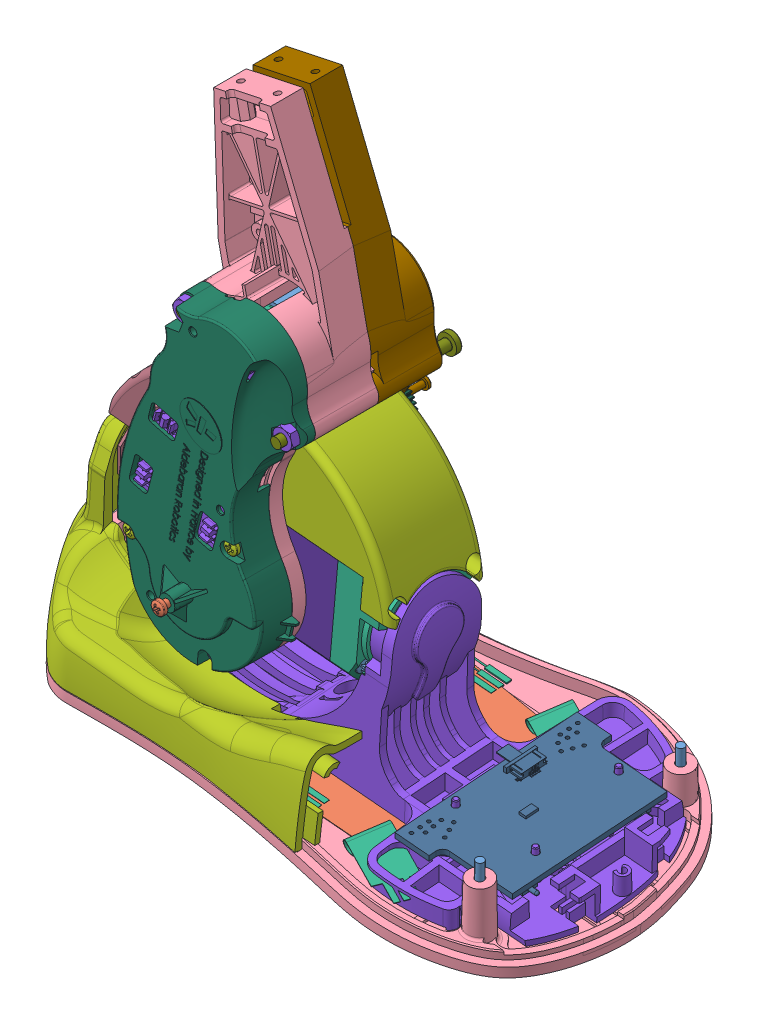
SolidWorks assembly Tibia_gauche, configuration Défaut. Lengths in mm.
Overall size (176.95 174.24 110.8).
97 component instances, 51 part files, 74 mates.
Components (placement in the parent):
- STD_M700013__PZ99_KA22x5_KA22 x 6-1: STD_M700013__PZ99_KA22x5_KA22 x 6 [Default] at (16.9636 -10.9615 1.7353) x (0 0 1) z (0.337513 -0.941321 0) size (6.5 3.9 3.91)
- STD_M700003__PZ99_KA22x6_KA22 x 6-1: STD_M700003__PZ99_KA22x6_KA22 x 6 [Default] at (2.1457 -91.3172 43.0853) x (0 0 -1) z (0.448628 -0.893719 0) size (7.5 3.9 3.91)
- ALD_M010013__P_mobile_inf_1_A00-1: ALD_M010013__P_mobile_inf_1_A00 [Default] at (6.6023 -47.3511 -13.8647) x (-0.555489 0.831524 0) z (-0.831524 -0.555489 0) size (24.51 6.7 24.51)
- ALD_M010048__P_couvercle_tibia_meca_gauche_Axx-1: ALD_M010048__P_couvercle_tibia_meca_gauche_Axx [Default] at (2.8538 9.7275 -12.4647) x (0 -1 0) z (0 0 1) size (91.48 47.32 23.1) (hidden)
- ALD_M010046__P_boitier_tibia_elec_gauche_ALD_M010046__PAxx_boitier_elec_gauche-1: ALD_M010046__P_boitier_tibia_elec_gauche_ALD_M010046__PAxx_boitier_elec_gauche [Default] at (2.8538 9.7275 5.2353) x (0 -1 0) z (0 0 1) size (135.22 47.39 29.9)
- STD_M700013__PZ99_KA22x5_KA22 x 6-2: STD_M700013__PZ99_KA22x5_KA22 x 6 [Default] at (-1.6212 -14.9118 1.7353) x (0 0 1) z (-0.935228 -0.354047 0) size (6.5 3.9 3.91)
- STD_M710004__P_vis_M2x5_ALD_M710004__PZ99_vis_M2x5-1: STD_M710004__P_vis_M2x5_ALD_M710004__PZ99_vis_M2x5 [Default] at (10.4845 -27.6822 -14.6647) x (0 0 1) z (0.702902 0.711287 0) size (6.41 3.8 3.8)
- ALD_M840031-1: ALD_M840031 [Default] at (12.0374 -33.4777 18.7353) x (-0.707107 -0.707107 0) z (0.707107 -0.707107 0) size (22 50.65 22)
- STD_M700005__PZ99_KA22x12_Default-1: STD_M700005__PZ99_KA22x12_Default [Default] at (14.3538 -74.4725 34.0353) x (0 0 -1) z (0.975434 -0.220294 0) size (13.5 3.9 3.91)
- STD_M710004__P_vis_M2x5_ALD_M710004__PZ99_vis_M2x5-2: STD_M710004__P_vis_M2x5_ALD_M710004__PZ99_vis_M2x5 [Default] at (17.8329 -35.0307 -14.6647) x (0 0 1) z (0.331606 0.943418 0) size (6.41 3.8 3.8)
- ALD_E000183__P_Left_Tibia_Card_Default-1: ALD_E000183__P_Left_Tibia_Card_Default [Default] at (-4.5707 -75.2219 31.3353) x (-0.250739 -0.968055 0) z (0 0 1) size (56.57 25 8.51)
- STD_M700006__PZ99_KA18x6_Default-1: STD_M700006__PZ99_KA18x6_Default [Default] at (-0.8831 -76.2311 -39.0647) x (0 0 1) z (0.79364 0.608388 0) size (7.2 3.2 3.2)
- STD_M510004__P_palier_GFM_1517-05_stabdard-1: STD_M510004__P_palier_GFM_1517-05_stabdard [Default] at (2.8538 -90.2725 -9.0647) x (0 0 -1) z (0.822457 -0.568828 0) size (5 23 23)
- ALD_M100068__P_Pinion_inf_4_A00-1: ALD_M100068__P_Pinion_inf_4_A00 [Default] at (-2.245 -74.58 -24.3647) x (0.042959 -0.999077 0) z (-0.999077 -0.042959 0) size (8.58 10.5 8.96)
- ALD_M010289__P_Inf_Limiter_Default-1: ALD_M010289__P_Inf_Limiter_Default [Default] at (-2.245 -74.58 -24.4647) x (0.999077 0.042959 0) z (0 0 1) size (16.14 19.2 3.9)
- STD_M510004__P_palier_GFM_1517-05_stabdard-2: STD_M510004__P_palier_GFM_1517-05_stabdard [Default] at (2.8538 -90.2725 19.5353) x (0 0 1) z (-0.611916 -0.790923 0) size (5 23 23)
- ALD_E000030__P_carte_MRE-1: ALD_E000030__P_carte_MRE [Default] at (-7.1462 -100.2725 30.9353) x (0 1 0) z (0 0 -1) size (18.94 18.94 5)
- ALD_M100018__P_axe_3x20_2-1: ALD_M100018__P_axe_3x20_2 [Default] at (-2.245 -74.58 -29.5647) x (-0.898721 -0.43852 0) z (0 0 1) size (3 3 20)
- ALD_M010050__P_couvercle_tibia_elec_gauche_Axx-1: ALD_M010050__P_couvercle_tibia_elec_gauche_Axx [Default] at (3.2067 9.6772 24.5353) x (-0.010505 -0.999945 0) z (0 0 1) size (91.58 50.24 17.3)
- STD_M700005__PZ99_KA22x12_Default-2: STD_M700005__PZ99_KA22x12_Default [Default] at (-15.1462 -84.8725 -22.6647) x (0 0 1) z (-0.865979 -0.500081 0) size (13.5 3.9 3.91)
- STD_M710005__PZ99_Vis_M3x50_ISO 7045 - M3 x 50-1: STD_M710005__PZ99_Vis_M3x50_ISO 7045 - M3 x 50 [Default] at (-1.7576 -23.8893 -20.5647) x (0 0 1) z (0.06312 0.998006 0) size (52.4 5.6 5.68)
- ALD_M010014__P_mobile_inf_2_A00-1: ALD_M010014__P_mobile_inf_2_A00 [Default] at (1.2276 -60.6565 -18.3647) x (0.438964 -0.898505 0) z (0.898505 0.438964 0) size (19.63 8.2 19.62)
- Left_Foot_jambe droite-1: Left_Foot_jambe droite [Défaut] at (4.3479 -90.4053 5.2353) x (-0.007082 -0.079671 0.996796) z (-0.996073 0.088539 0) size (106.44 58.7 171.69)
  - STD_M850001__P_Scotch_double_Face_3M_5419_Default-1: STD_M850001__P_Scotch_double_Face_3M_5419_Default [Default] at (-23.9002 -40.8442 -61.9998) x (0 0 -1) z (0 1 0) size (13 10 0.25)
  - STD_M700004__PZ99_KA22x8_KA22 x 8-1: STD_M700004__PZ99_KA22x8_KA22 x 8 [Default] at (-16.4 -30.0842 45.1) x (0 1 0) z (-0.943584 0 -0.331134) size (9.5 3.9 3.91)
  - STD_M850001__P_Scotch_double_Face_3M_5419_Default-2: STD_M850001__P_Scotch_double_Face_3M_5419_Default [Default] at (27.1002 -40.5942 -74.9998) x (0 0 1) z (0 -1 0) size (13 10 0.25)
  - STD_E990013__P_FSR_4P-1: STD_E990013__P_FSR_4P [Default] at (19.0956 -40.8442 30.9044) x (0 0 1) z (0 -1 0) size (108.1 14 0.37)
  - STD_M700004__PZ99_KA22x8_KA22 x 8-2: STD_M700004__PZ99_KA22x8_KA22 x 8 [Default] at (13.2 -30.0842 45.1) x (0 1 0) z (-0.676128 0 -0.736784) size (9.5 3.9 3.91)
  - STD_M830010__P_Axial_Magnet_6x3_Default-1: STD_M830010__P_Axial_Magnet_6x3_Default [Default] at (-0.0436 -43.3342 -16.4801) x (0.495785 0 -0.868445) z (0 1 0) size (6 6 3.01)
  - ALD_M010097__P_semelle_gauche_default-1: ALD_M010097__P_semelle_gauche_default [Default] at (0 -45.0842 21.6) x (0 0 -1) z (0 1 0) size (171.69 106.44 28.07)
  - STD_M850001__P_Scotch_double_Face_3M_5419_Default-3: STD_M850001__P_Scotch_double_Face_3M_5419_Default [Default] at (-24.4459 -40.8442 37.9999) x (0.087156 0 -0.996195) z (0 1 0) size (13 10 0.25)
  - STD_M510003__P_palier_GFM_1012-07_stabdard-1: STD_M510003__P_palier_GFM_1012-07_stabdard [Default] at (0 0 31.4) x (0 0 1) z (-0.219796 0.975546 0) size (7 18 18)
  - STD_M850001__P_Scotch_double_Face_3M_5419_Default-4: STD_M850001__P_Scotch_double_Face_3M_5419_Default [Default] at (13.1002 -40.8442 36.8998) x (1 0 0) z (0 1 0) size (13 10 0.25)
  - STD_E990012__P_FSR_2P_pli 4-1: STD_E990012__P_FSR_2P_pli 4 [Default] at (23.0956 -40.8442 -69.0044) x (0 0 -1) z (0 -1 0) size (57.3 20.1 4.54)
  - ALD_M010133__P_coque_interieure_pied_gauche-1: ALD_M010133__P_coque_interieure_pied_gauche [Default] at (0 -45.0842 21.6) x (0 0 -1) z (0 1 0) size (104.04 41.95 56.84)
  - STD_M700004__PZ99_KA22x8_KA22 x 8-3: STD_M700004__PZ99_KA22x8_KA22 x 8 [Default] at (-4.25 -31.212 18.3352) x (0 0 1) z (0.021347 -0.999772 0) size (9.5 3.9 3.91)
  - ALD_M010099__P_structure_pied_gauche_default-1: ALD_M010099__P_structure_pied_gauche_default [Default] at (-6.6116 -41.5942 -17.9596) x (0 1 0) z (0 0 -1) size (54.34 78.21 137.68)
  - STD_M700004__PZ99_KA22x8_KA22 x 8-4: STD_M700004__PZ99_KA22x8_KA22 x 8 [Default] at (4.25 -31.212 18.3521) x (0 0 1) z (0.183952 -0.982935 0) size (9.5 3.9 3.91)
  - ALD_M010018__P_support_dente_A08-1: ALD_M010018__P_support_dente_A08 [Default] at (0 0 31.2) x (0 0 -1) z (-1 0 0) size (20.4 48.62 27.24)
  - STD_M700004__PZ99_KA22x8_KA22 x 8-5: STD_M700004__PZ99_KA22x8_KA22 x 8 [Default] at (26.7 -30.0842 -81.8) x (0 1 0) z (-0.96573 0 -0.25955) size (9.5 3.9 3.91)
  - STD_M700004__PZ99_KA22x8_KA22 x 8-6: STD_M700004__PZ99_KA22x8_KA22 x 8 [Default] at (-31.7 -35.0842 -81.8) x (0 1 0) z (-0.841418 0 -0.540385) size (9.5 3.9 3.91)
  - STD_M830010__P_Axial_Magnet_6x3_Default-2: STD_M830010__P_Axial_Magnet_6x3_Default [Default] at (-0.0436 -39.0942 -16.4801) x (-0.919248 0 0.393679) z (0 1 0) size (6 6 3.01)
  - STD_E990013__P_FSR_4P-2: STD_E990013__P_FSR_4P [Default] at (-29.896 -40.8442 31.5047) x (-0.087156 0 0.996195) z (0 -1 0) size (108.1 14 0.37)
  - ALD_E000030__P_carte_MRE-1: ALD_E000030__P_carte_MRE [Default] at (10 10 41.9) x (0 -1 0) z (0 0 -1) size (18.94 18.94 5)
  - STD_E990012__P_FSR_2P_pli 4-2: STD_E990012__P_FSR_2P_pli 4 [Default] at (-29.8956 -40.8442 -69.0068) x (0 0 -1) z (0 -1 0) size (57.3 20.1 4.54)
  - ALD_E000032__P_Carte_Moteur_Pied_A00-1: ALD_E000032__P_Carte_Moteur_Pied_A00 [Default] at (19.9576 -32.4942 -54.2074) size (53 5.6 34.31)
- Left_Ankle_X_DOF_type I-1: Left_Ankle_X_DOF_type I [Défaut] at (72.1207 -93.7188 5.2353) x (0 0 1) z (-0.996073 0.088539 0) size (56.71 61.38 84.83)
  - STD_M700004__PZ99_KA22x8_KA22 x 8-1: STD_M700004__PZ99_KA22x8_KA22 x 8 [Default] at (11.35 24.8 98.9) x (0 0 -1) z (0.764659 -0.644435 0) size (9.5 3.9 3.91)
  - ALD_M100016__P_axe_3x27_3-1: ALD_M100016__P_axe_3x27_3 [Default] at (0 13.8 108.25) x (0.974112 0.226065 0) z (0 0 -1) size (3 3 27.3)
  - STD_M700004__PZ99_KA22x8_KA22 x 8-2: STD_M700004__PZ99_KA22x8_KA22 x 8 [Default] at (11.35 -11.2 98.9) x (0 0 -1) z (0.336461 0.941697 0) size (9.5 3.9 3.91)
  - STD_M700004__PZ99_KA22x8_KA22 x 8-3: STD_M700004__PZ99_KA22x8_KA22 x 8 [Default] at (0 -14.2 98.9) x (0 0 -1) z (0.992514 -0.122129 0) size (9.5 3.9 3.91)
  - ALD_M010014__P_mobile_inf_2_A00-1: ALD_M010014__P_mobile_inf_2_A00 [Default] at (0 -0.6 88.9) x (-0.518728 -0.854939 0) z (-0.854939 0.518728 0) size (19.63 8.2 19.62)
  - STD_M700004__PZ99_KA22x8_KA22 x 8-4: STD_M700004__PZ99_KA22x8_KA22 x 8 [Default] at (-11.35 -11.2 98.9) x (0 0 -1) z (0.352099 0.935963 0) size (9.5 3.9 3.91)
  - ALD_M100067__P_Pinion_Inf_3_A00-1: ALD_M100067__P_Pinion_Inf_3_A00 [Default] at (0 13.8 92.9) x (-0.113825 -0.993501 0) z (-0.993501 0.113825 0) size (8.58 13 8.96)
  - ALD_M010033__P_couvercle_X_AV_cheville_A02-1: ALD_M010033__P_couvercle_X_AV_cheville_A02 [Default] at (-14.1 0 81) x (0 0 1) z (-1 0 0) size (18.62 54.33 28.93)
  - STD_M700002__P_KA22x14-1: STD_M700002__P_KA22x14 [Default] at (11.1 8.9613 30.2) x (0 0 1) z (-1 0 0) size (15.5 3.9 3.91)
  - ALD_M010288__P_Inf_Wheel_3&4_A00-1: ALD_M010288__P_Inf_Wheel_3&4_A00 [Default] at (0 13.8 91.2) x (-0.969302 -0.245872 0) z (-0.245872 0.969302 0) size (24.52 5.6 24.55)
  - ALD_M100015__P_axe_2x13-1: ALD_M100015__P_axe_2x13 [Default] at (0 -0.6 100.1) x (-0.263366 -0.964696 0) z (0 0 -1) size (2 2 13)
  - ALD_M010030__P_cage_fut_moteur_cheville_gauche_Axx-1: ALD_M010030__P_cage_fut_moteur_cheville_gauche_Axx [Default] at origin size (43 61.38 54.3)
  - ALD_M100004__P_axe_Y_B00-1: ALD_M100004__P_axe_Y_B00 [Default] at (-15.4 -2.7 69.3) x (0 -0.999499 -0.031657) z (0 0.031657 -0.999499) size (4 18.6 4)
  - STD_M710004__P_vis_M2x5_ALD_M710004__PZ99_vis_M2x5-1: STD_M710004__P_vis_M2x5_ALD_M710004__PZ99_vis_M2x5 [Default] at (4.9149 -3.4415 83.9) x (0 0 -1) z (-0.816228 0.57773 0) size (6.41 3.8 3.8)
  - ALD_E000030__P_carte_MRE-1: ALD_E000030__P_carte_MRE [Default] at (10 10 39) x (-1 0 0) z (0 0 1) size (18.94 18.94 5)
  - ALD_M010292__P_Motor_Ring_Default-1: ALD_M010292__P_Motor_Ring_Default [Default] at (0 0 51.8) x (0.930686 0.365818 0) z (0 0 1) size (24 24 29.5)
  - ALD_M010289__P_Inf_Limiter_Default-1: ALD_M010289__P_Inf_Limiter_Default [Default] at (0 13.8 92.8) x (0.993501 -0.113825 0) z (0 0 1) size (16.14 19.2 3.9)
  - ALD_M080003__P_rondelle_flex_X_cheville_A00-1: ALD_M080003__P_rondelle_flex_X_cheville_A00 [Default] at (0 -2.7 27.95) size (16 16 0.25)
  - ALD_M010013__P_mobile_inf_1_A00-1: ALD_M010013__P_mobile_inf_1_A00 [Default] at (0 13.8 84.4) x (0.2094 0.97783 0) z (0.97783 -0.2094 0) size (24.51 6.7 24.51)
  - STD_M710004__P_vis_M2x5_ALD_M710004__PZ99_vis_M2x5-2: STD_M710004__P_vis_M2x5_ALD_M710004__PZ99_vis_M2x5 [Default] at (-4.9149 3.4415 83.9) x (0 0 -1) z (-0.989398 0.145226 0) size (6.41 3.8 3.8)
  - ALD_M840030__P_Portescap_22NT_82_213P_Z13_Default-1: ALD_M840030__P_Portescap_22NT_82_213P_Z13_Default [Default] at (0 0 51.3) x (-0.906308 -0.422618 0) z (-0.422618 0.906308 0) size (22 50.65 22)
  - STD_M710004__P_vis_M2x5_ALD_M710004__PZ99_vis_M2x5-3: STD_M710004__P_vis_M2x5_ALD_M710004__PZ99_vis_M2x5 [Default] at (5.4378 2.5357 83.9) x (0 0 -1) z (0.998872 -0.04749 0) size (6.41 3.8 3.8)
  - ALD_M010053__P_support_aimant-1: ALD_M010053__P_support_aimant [Default] at (0 0 48.9) x (-0.941844 0.33605 0) z (-0.33605 -0.941844 0) size (7.64 6.4 7.6)
  - STD_M700004__PZ99_KA22x8_KA22 x 8-5: STD_M700004__PZ99_KA22x8_KA22 x 8 [Default] at (11.35 -11.2 34.7) x (0 0 1) z (0.583852 -0.81186 0) size (9.5 3.9 3.91)
  - ALD_M010053__P_support_aimant-2: ALD_M010053__P_support_aimant [Default] at (0 -2.7 100.8) x (-0.5 -0.866025 0) z (-0.866025 0.5 0) size (7.64 6.4 7.6)
  - STD_M700004__PZ99_KA22x8_KA22 x 8-6: STD_M700004__PZ99_KA22x8_KA22 x 8 [Default] at (-11.35 -11.2 34.7) x (0 0 1) z (0.983779 0.179385 0) size (9.5 3.9 3.91)
  - ALD_M010201__P_magnet_wires_support-1: ALD_M010201__P_magnet_wires_support [Default] at (16.3 -2.7 69.3) x (0 0 -1) z (0 -1 0) size (14 6.41 14)
  - STD_M700002__P_KA22x14-2: STD_M700002__P_KA22x14 [Default] at (-11.1 8.9613 30.2) x (0 0 1) z (0.995485 0.094917 0) size (15.5 3.9 3.91)
  - STD_M700004__PZ99_KA22x8_KA22 x 8-7: STD_M700004__PZ99_KA22x8_KA22 x 8 [Default] at (0 -14.2 34.7) x (0 0 1) z (0.928947 -0.370213 0) size (9.5 3.9 3.91)
  - ALD_M010035__P_couvercle_X_AR_Axx-1: ALD_M010035__P_couvercle_X_AR_Axx [Default] at (0 0 42.7) x (-1 0 0) z (0 0 -1) size (28.83 33.93 15.89)
  - STD_M700004__PZ99_KA22x8_KA22 x 8-8: STD_M700004__PZ99_KA22x8_KA22 x 8 [Default] at (-11.35 24.8 98.9) x (0 0 -1) z (0.765986 -0.642858 0) size (9.5 3.9 3.91)
  - ALD_M010055__P_cache_fut_moteur_cheville_A-1: ALD_M010055__P_cache_fut_moteur_cheville_A [Default] at (14.1 0 0) x (0 0 -1) z (1 0 0) size (45.42 37.32 28.46)
- STD_M700005__PZ99_KA22x12_Default-3: STD_M700005__PZ99_KA22x12_Default [Default] at (-15.1462 -84.8725 34.0353) x (0 0 -1) z (-0.568693 -0.82255 0) size (13.5 3.9 3.91)
- STD_M710002__P_ecrou_M3-1: STD_M710002__P_ecrou_M3 [Default] at (25.8324 -43.0662 29.9353) x (0.734221 -0.678911 0) z (0 0 1) size (5.5 6.35 2.4)
- STD_M700005__PZ99_KA22x12_Default-4: STD_M700005__PZ99_KA22x12_Default [Default] at (-12.1462 -61.8725 -22.6647) x (0 0 1) z (-0.987069 0.160297 0) size (13.5 3.9 3.91)
- ALD_M010288__P_Inf_Wheel_3&4_A00-1: ALD_M010288__P_Inf_Wheel_3&4_A00 [Default] at (-2.245 -74.58 -25.8647) x (0.367326 -0.930092 0) z (-0.930092 -0.367326 0) size (24.52 5.6 24.55)
- STD_M710005__PZ99_Vis_M3x50_ISO 7045 - M3 x 50-2: STD_M710005__PZ99_Vis_M3x50_ISO 7045 - M3 x 50 [Default] at (25.8324 -43.0662 -20.5647) x (0 0 1) z (-0.935181 -0.354169 0) size (52.4 5.6 5.68)
- STD_M700005__PZ99_KA22x12_Default-5: STD_M700005__PZ99_KA22x12_Default [Default] at (5.8538 -107.2725 -22.6647) x (0 0 1) z (0.139397 0.990237 0) size (13.5 3.9 3.91)
- ALD_M010292__P_Motor_Ring_Default-1: ALD_M010292__P_Motor_Ring_Default [Default] at (12.0374 -33.4777 -11.2647) x (0.565934 0.824451 0) z (0 0 1) size (24 24 29.5)
- ALD_M010044__P_boitier_tibia_meca_gauche_ALD_M010044__PAxx_boitier_tibia_meca_gauche-1: ALD_M010044__P_boitier_tibia_meca_gauche_ALD_M010044__PAxx_boitier_tibia_meca_gauche [Default] at (2.8538 9.7275 5.2353) x (0 -1 0) z (0 0 1) size (135.22 47.39 25.5)
- STD_M510002__P_palier_GSM_0405-04-1: STD_M510002__P_palier_GSM_0405-04 [Default] at (2.8538 -90.2725 -28.7647) x (0.409552 -0.912287 0) z (0 0 1) size (5.5 5.5 4)
- ALD_M100021__P_axe_3x11_7-1: ALD_M100021__P_axe_3x11_7 [Default] at (6.6023 -47.3511 -22.7647) x (-0.979613 0.200892 0) z (0 0 1) size (3 3 11.7)
- ALD_M010053__P_support_aimant-1: ALD_M010053__P_support_aimant [Default] at (12.0374 -33.4777 20.4853) x (0.99932 -0.036877 0) z (-0.036877 -0.99932 0) size (7.64 6.4 7.6)
- STD_M710004__P_vis_M2x5_ALD_M710004__PZ99_vis_M2x5-3: STD_M710004__P_vis_M2x5_ALD_M710004__PZ99_vis_M2x5 [Default] at (6.2418 -31.9248 -14.6647) x (0 0 1) z (-0.85095 0.525247 0) size (6.41 3.8 3.8)
- ALD_M100017__P_axe_2x19_7-1: ALD_M100017__P_axe_2x19_7 [Default] at (1.2276 -60.6565 -29.2647) x (-0.661597 -0.749859 0) z (0 0 1) size (2 2 19.7)
- STD_M710002__P_ecrou_M3-2: STD_M710002__P_ecrou_M3 [Default] at (-1.7576 -23.8893 31.4353) x (-0.847827 0.530273 0) z (0 0 1) size (5.5 6.35 2.4)
- STD_M700004__PZ99_KA22x8_KA22 x 8-2: STD_M700004__PZ99_KA22x8_KA22 x 8 [Default] at (5.8538 -107.2725 30.5353) x (0 0 -1) z (0.402889 -0.915249 0) size (9.5 3.9 3.91)
- STD_M700005__PZ99_KA22x12_Default-6: STD_M700005__PZ99_KA22x12_Default [Default] at (14.3538 -74.4725 -22.6647) x (0 0 1) z (0.865979 0.500081 0) size (13.5 3.9 3.91)
- ALD_M010016__P_roue_sortie_inf-1: ALD_M010016__P_roue_sortie_inf [Default] at (2.8538 -90.2725 -14.6647) x (-0.641723 0.766936 0) z (-0.766936 -0.641723 0) size (27.24 12.9 27.24)
- ALD6667-1: ALD6667 [Default] at (12.0374 -33.4777 -12.6647) x (-0.191867 -0.981421 0) z (0.981421 -0.191867 0) size (6.6 3.4 6.59)
Mates (geometry in assembly coordinates):
- Coaxiale10: concentric aligned: cylinder of ALD_M010046__P_boitier_tibia_elec_gauche_ALD_M010046__PAxx_boitier_elec_gauche-1 through (8.3147 -27.3018 33.2353) axis (0 0 -1) radius 0.7501; cylinder of ALD_E000183__P_Left_Tibia_Card_Default-1 through (8.3147 -27.3018 29.7426) axis (0 0 -1) radius 0.775
- Coaxiale11: concentric aligned: cylinder of ALD_M010046__P_boitier_tibia_elec_gauche_ALD_M010046__PAxx_boitier_elec_gauche-1 through (2.8538 -90.2725 24.7353) axis (0 0 -1) radius 8.5; cylinder of STD_M510004__P_palier_GFM_1517-05_stabdard-2 through (2.8538 -90.2725 -980.4647) axis (0 0 -1) radius 8.5
- Coïncidente8: coincident anti-aligned: plane of ALD_M010046__P_boitier_tibia_elec_gauche_ALD_M010046__PAxx_boitier_elec_gauche-1 through (2.8538 -90.2725 20.5353) normal (0 0 -1); plane of STD_M510004__P_palier_GFM_1517-05_stabdard-2 through (-3.869 -85.0712 20.5353) normal (0 0 1)
- Coaxiale12: concentric anti-aligned: cone of ALD_M010046__P_boitier_tibia_elec_gauche_ALD_M010046__PAxx_boitier_elec_gauche-1 through (9.3538 -90.2725 30.1353) axis (0 0 1); cylinder of ALD_E000030__P_carte_MRE-1 through (9.3538 -90.2725 30.9353) axis (0 0 -1) radius 1.25
- Coaxiale13: concentric anti-aligned: cone of ALD_M010046__P_boitier_tibia_elec_gauche_ALD_M010046__PAxx_boitier_elec_gauche-1 through (-3.6462 -90.2725 30.1353) axis (0 0 1); cylinder of ALD_E000030__P_carte_MRE-1 through (-3.6462 -90.2725 30.9353) axis (0 0 -1) radius 1.25
- Coïncidente9: coincident anti-aligned: plane of ALD_M010046__P_boitier_tibia_elec_gauche_ALD_M010046__PAxx_boitier_elec_gauche-1 through (-18.7219 -89.2094 30.1353) normal (0 0 1); plane of ALD_E000030__P_carte_MRE-1 through (2.8538 -90.2725 30.1353) normal (0 0 -1)
- Coaxiale16: concentric anti-aligned: cone of ALD_M010046__P_boitier_tibia_elec_gauche_ALD_M010046__PAxx_boitier_elec_gauche-1 through (-1.7576 -23.8893 24.7353) axis (0 0 -1); cylinder of STD_M710002__P_ecrou_M3-2 through (-1.7576 -23.8893 29.0353) axis (0 0 1) radius 1.25
- Coaxiale35: concentric aligned: cylinder of ALD_M100068__P_Pinion_inf_4_A00-1 through (-2.245 -74.58 -24.3647) axis (0 0 -1) radius 1.5; cylinder of ALD_M100018__P_axe_3x20_2-1 through (-2.245 -74.58 -9.5647) axis (0 0 -1) radius 1.5
- Coïncidente39: coincident anti-aligned: plane of ALD_M100068__P_Pinion_inf_4_A00-1 through (-1.8674 -71.9925 -36.7693) normal (-0.106906 0.994269 0); plane of ALD_M010289__P_Inf_Limiter_Default-1 through (0.8247 -71.703 -24.4647) normal (0.106906 -0.994269 0)
- Coaxiale42: concentric aligned: circle of ALD_M100068__P_Pinion_inf_4_A00-1; circle of ALD_M010289__P_Inf_Limiter_Default-1
- Coïncidente40: coincident anti-aligned: plane of ALD_M100068__P_Pinion_inf_4_A00-1 through (-2.245 -74.58 -20.5647) normal (0 0 -1); plane of ALD_M010289__P_Inf_Limiter_Default-1 through (-2.245 -74.58 -20.5647) normal (0 0 1)
- Coaxiale43: concentric aligned: cylinder of ALD_M100018__P_axe_3x20_2-1 through (-2.245 -74.58 -9.5647) axis (0 0 -1) radius 1.5; cylinder of ALD_M010288__P_Inf_Wheel_3&4_A00-1 through (-2.245 -74.58 -25.8647) axis (0 0 -1) radius 1.5
- Coïncidente41: coincident anti-aligned: plane of ALD_M010289__P_Inf_Limiter_Default-1 through (-2.245 -74.58 -24.4647) normal (0 0 -1); plane of ALD_M010288__P_Inf_Wheel_3&4_A00-1 through (1.7717 -84.7506 -24.4647) normal (0 0 1)
- Coaxiale44: concentric aligned: cone of ALD_M010046__P_boitier_tibia_elec_gauche_ALD_M010046__PAxx_boitier_elec_gauche-1 through (25.8324 -43.0662 22.4353) axis (0 0 -1); cylinder of STD_M710005__PZ99_Vis_M3x50_ISO 7045 - M3 x 50-2 through (25.8324 -43.0662 -45.9647) axis (0 0 -1) radius 1.5
- Coaxiale45: concentric aligned: cone of ALD_M010046__P_boitier_tibia_elec_gauche_ALD_M010046__PAxx_boitier_elec_gauche-1 through (-1.7576 -23.8893 24.7353) axis (0 0 -1); cylinder of STD_M710005__PZ99_Vis_M3x50_ISO 7045 - M3 x 50-1 through (-1.7576 -23.8893 -45.9647) axis (0 0 -1) radius 1.5
- Coaxiale46: concentric aligned: cylinder of ALD_M010050__P_couvercle_tibia_elec_gauche_Axx-1 through (25.8324 -43.0662 35.0235) axis (0 0 -1) radius 1.6; cylinder of STD_M710005__PZ99_Vis_M3x50_ISO 7045 - M3 x 50-2 through (25.8324 -43.0662 -45.9647) axis (0 0 -1) radius 1.5
- Coaxiale47: concentric aligned: cylinder of ALD_M010050__P_couvercle_tibia_elec_gauche_Axx-1 through (-1.7576 -23.8893 39.0608) axis (0 0 -1) radius 1.6; cylinder of STD_M710005__PZ99_Vis_M3x50_ISO 7045 - M3 x 50-1 through (-1.7576 -23.8893 -45.9647) axis (0 0 -1) radius 1.5
- Coïncidente43: coincident anti-aligned: plane of ALD_M010046__P_boitier_tibia_elec_gauche_ALD_M010046__PAxx_boitier_elec_gauche-1 through (5.6349 -42.4232 23.7353) normal (0 0 1); plane of ALD_M010050__P_couvercle_tibia_elec_gauche_Axx-1 through (-12.8867 -31.5309 23.7353) normal (0 0 -1)
- Coïncidente44: coincident anti-aligned: plane of ALD_M010050__P_couvercle_tibia_elec_gauche_Axx-1 through (35.0516 -51.7138 27.5353) normal (0 0 1); plane of STD_M710002__P_ecrou_M3-1 through (27.9882 -40.7347 27.5353) normal (0 0 -1)
- Coaxiale48: concentric anti-aligned: cylinder of STD_M710002__P_ecrou_M3-1 through (25.8324 -43.0662 27.5353) axis (0 0 1) radius 1.25; cylinder of STD_M710005__PZ99_Vis_M3x50_ISO 7045 - M3 x 50-2 through (25.8324 -43.0662 -45.9647) axis (0 0 -1) radius 1.5
- Coaxiale49: concentric anti-aligned: cylinder of ALD_M010050__P_couvercle_tibia_elec_gauche_Axx-1 through (-15.1462 -84.8725 39.0608) axis (0 0 -1) radius 1.25; cylinder of STD_M700005__PZ99_KA22x12_Default-3 through (-15.1462 -84.8725 59.4353) axis (0 0 1) radius 1.1
- Coïncidente48: coincident anti-aligned: plane of ALD_M010050__P_couvercle_tibia_elec_gauche_Axx-1 through (5.8538 -107.2725 32.5353) normal (0 0 1); plane of STD_M700005__PZ99_KA22x12_Default-3 through (-14.2414 -85.498 32.5353) normal (0 0 -1)
- Coaxiale50: concentric anti-aligned: cone of ALD_M010050__P_couvercle_tibia_elec_gauche_Axx-1 through (5.8538 -107.2725 32.5353) axis (0 0 -1); cylinder of STD_M700004__PZ99_KA22x8_KA22 x 8-2 through (5.8538 -107.2725 55.9353) axis (0 0 1) radius 1.1
- Coïncidente49: coincident anti-aligned: plane of ALD_M010050__P_couvercle_tibia_elec_gauche_Axx-1 through (5.8538 -107.2725 29.0353) normal (0 0 1); plane of STD_M700004__PZ99_KA22x8_KA22 x 8-2 through (6.8606 -106.8293 29.0353) normal (0 0 -1)
- Coaxiale51: concentric anti-aligned: cylinder of STD_M700005__PZ99_KA22x12_Default-1 through (14.3538 -74.4725 59.4353) axis (0 0 1) radius 1.1; cylinder of ALD_M010050__P_couvercle_tibia_elec_gauche_Axx-1 through (14.3538 -74.4725 39.0608) axis (0 0 -1) radius 1.25
- Coïncidente50: coincident anti-aligned: plane of STD_M700005__PZ99_KA22x12_Default-1 through (14.5961 -73.3995 32.5353) normal (0 0 -1); plane of ALD_M010050__P_couvercle_tibia_elec_gauche_Axx-1 through (14.3538 -74.4725 32.5353) normal (0 0 1)
- Coïncidente51: coincident anti-aligned: plane of ALD_M010050__P_couvercle_tibia_elec_gauche_Axx-1 through (0.2578 -26.3431 29.0353) normal (0 0 1); plane of STD_M710002__P_ecrou_M3-2 through (-3.4415 -26.5815 29.0353) normal (0 0 -1)
- Coïncidente52: coincident anti-aligned: plane of ALD_M010048__P_couvercle_tibia_meca_gauche_Axx-1 through (29.6697 -56.0093 -18.1647) normal (0 0 -1); plane of STD_M710005__PZ99_Vis_M3x50_ISO 7045 - M3 x 50-2 through (25.3011 -41.6634 -18.1647) normal (0 0 1)
- Coaxiale53: concentric aligned: cone of ALD_M010048__P_couvercle_tibia_meca_gauche_Axx-1 through (25.8324 -43.0662 -14.0647) axis (0 0 -1); cylinder of STD_M710005__PZ99_Vis_M3x50_ISO 7045 - M3 x 50-2 through (25.8324 -43.0662 -45.9647) axis (0 0 -1) radius 1.5
- Coaxiale55: concentric anti-aligned: cylinder of ALD_M010048__P_couvercle_tibia_meca_gauche_Axx-1 through (2.8538 -90.2725 -29.8647) axis (0 0 1) radius 2.75; cylinder of STD_M510002__P_palier_GSM_0405-04-1 through (2.8538 -90.2725 -24.7647) axis (0 0 -1) radius 2.75
- Coïncidente54: coincident anti-aligned: plane of ALD_M010048__P_couvercle_tibia_meca_gauche_Axx-1 through (2.8538 -90.2725 -28.7647) normal (0 0 1); plane of STD_M510002__P_palier_GSM_0405-04-1 through (2.8538 -90.2725 -28.7647) normal (0 0 -1)
- Coaxiale56: concentric aligned: cone of ALD_M010048__P_couvercle_tibia_meca_gauche_Axx-1 through (-1.7576 -23.8893 -14.0647) axis (0 0 -1); cylinder of STD_M710005__PZ99_Vis_M3x50_ISO 7045 - M3 x 50-1 through (-1.7576 -23.8893 -45.9647) axis (0 0 -1) radius 1.5
- Coïncidente55: coincident anti-aligned: plane of ALD_M010048__P_couvercle_tibia_meca_gauche_Axx-1 through (29.6697 -56.0093 -18.1647) normal (0 0 -1); plane of STD_M710005__PZ99_Vis_M3x50_ISO 7045 - M3 x 50-1 through (-0.2606 -23.984 -18.1647) normal (0 0 1)
- Coïncidente56: coincident anti-aligned: plane of ALD_M010048__P_couvercle_tibia_meca_gauche_Axx-1 through (-12.1462 -61.8725 -21.1647) normal (0 0 -1); plane of STD_M700005__PZ99_KA22x12_Default-4 through (-11.9699 -60.7867 -21.1647) normal (0 0 1)
- Coïncidente57: coincident anti-aligned: plane of ALD_M010048__P_couvercle_tibia_meca_gauche_Axx-1 through (-15.1462 -84.8725 -21.1647) normal (0 0 -1); plane of STD_M700005__PZ99_KA22x12_Default-2 through (-15.6963 -83.9199 -21.1647) normal (0 0 1)
- Coïncidente58: coincident anti-aligned: plane of ALD_M010048__P_couvercle_tibia_meca_gauche_Axx-1 through (5.8538 -107.2725 -21.1647) normal (0 0 -1); plane of STD_M700005__PZ99_KA22x12_Default-5 through (6.9431 -107.4258 -21.1647) normal (0 0 1)
- Coïncidente59: coincident anti-aligned: plane of ALD_M010048__P_couvercle_tibia_meca_gauche_Axx-1 through (14.3538 -74.4725 -21.1647) normal (0 0 -1); plane of STD_M700005__PZ99_KA22x12_Default-6 through (14.9039 -75.4251 -21.1647) normal (0 0 1)
- Coaxiale69: concentric aligned: cylinder of STD_M510004__P_palier_GFM_1517-05_stabdard-1 through (2.8538 -90.2725 990.9353) axis (0 0 1) radius 7.5; cylinder of Left_Ankle_X_DOF_type I-1/ALD_M100004__P_axe_Y_B00-1 through (2.8538 -90.2725 989.8353) axis (0 0 1) radius 2
- Distance1: distance = 0.2 mm anti-aligned: plane of STD_M510004__P_palier_GFM_1517-05_stabdard-1 through (9.3953 -80.8142 -9.0647) normal (0 0 1); plane of Left_Ankle_X_DOF_type I-1/ALD_M010030__P_cage_fut_moteur_cheville_gauche_Axx-1 through (-21.9344 -98.075 -8.8647) normal (0 0 -1)
- Coaxiale71: concentric aligned: cylinder of Left_Foot_jambe droite-1/ALD_M010099__P_structure_pied_gauche_default-1 through (498058.5909 -44361.5126 5.2353) axis (-0.996073 0.088539 0) radius 9; cylinder of Left_Ankle_X_DOF_type I-1/ALD_M010035__P_couvercle_X_AR_Axx-1 through (43.7924 -93.9114 5.2353) axis (-0.996073 0.088539 0) radius 9
- Coïncidente69: coincident anti-aligned: plane of Left_Foot_jambe droite-1/ALD_M010099__P_structure_pied_gauche_default-1 through (38.812 -93.4687 5.2353) normal (-0.996073 0.088539 0); plane of Left_Ankle_X_DOF_type I-1/ALD_M010035__P_couvercle_X_AR_Axx-1 through (35.9276 -125.9189 5.2353) normal (0.996073 -0.088539 0)
- Verrouiller1: lock: unknown of ALD_M010046__P_boitier_tibia_elec_gauche_ALD_M010046__PAxx_boitier_elec_gauche-1; unknown of ALD_M010044__P_boitier_tibia_meca_gauche_ALD_M010044__PAxx_boitier_tibia_meca_gauche-1
- Verrouiller2: lock: unknown of STD_M710005__PZ99_Vis_M3x50_ISO 7045 - M3 x 50-2; unknown of ALD_M010044__P_boitier_tibia_meca_gauche_ALD_M010044__PAxx_boitier_tibia_meca_gauche-1
- Verrouiller3: lock: unknown of STD_M710005__PZ99_Vis_M3x50_ISO 7045 - M3 x 50-1; unknown of ALD_M010044__P_boitier_tibia_meca_gauche_ALD_M010044__PAxx_boitier_tibia_meca_gauche-1
- Verrouiller4: lock: unknown of STD_M710004__P_vis_M2x5_ALD_M710004__PZ99_vis_M2x5-1; unknown of ALD_M010044__P_boitier_tibia_meca_gauche_ALD_M010044__PAxx_boitier_tibia_meca_gauche-1
- Verrouiller5: lock: unknown of STD_M710004__P_vis_M2x5_ALD_M710004__PZ99_vis_M2x5-2; unknown of ALD_M010044__P_boitier_tibia_meca_gauche_ALD_M010044__PAxx_boitier_tibia_meca_gauche-1
- Verrouiller6: lock: unknown of ALD_M010044__P_boitier_tibia_meca_gauche_ALD_M010044__PAxx_boitier_tibia_meca_gauche-1; unknown of STD_M710004__P_vis_M2x5_ALD_M710004__PZ99_vis_M2x5-3
- Verrouiller7: lock: unknown of STD_M700005__PZ99_KA22x12_Default-5; unknown of ALD_M010044__P_boitier_tibia_meca_gauche_ALD_M010044__PAxx_boitier_tibia_meca_gauche-1
- Verrouiller8: lock: unknown of STD_M700005__PZ99_KA22x12_Default-2; unknown of ALD_M010044__P_boitier_tibia_meca_gauche_ALD_M010044__PAxx_boitier_tibia_meca_gauche-1
- Verrouiller10: lock: unknown of STD_M700005__PZ99_KA22x12_Default-4; unknown of ALD_M010044__P_boitier_tibia_meca_gauche_ALD_M010044__PAxx_boitier_tibia_meca_gauche-1
- Verrouiller11: lock: unknown of ALD_M010044__P_boitier_tibia_meca_gauche_ALD_M010044__PAxx_boitier_tibia_meca_gauche-1; unknown of STD_M700005__PZ99_KA22x12_Default-6
- Verrouiller12: lock: unknown of ALD_M100018__P_axe_3x20_2-1; unknown of ALD_M010044__P_boitier_tibia_meca_gauche_ALD_M010044__PAxx_boitier_tibia_meca_gauche-1
- Verrouiller13: lock: unknown of ALD_M010044__P_boitier_tibia_meca_gauche_ALD_M010044__PAxx_boitier_tibia_meca_gauche-1; unknown of ALD_M100017__P_axe_2x19_7-1
- Verrouiller14: lock: unknown of ALD_M010044__P_boitier_tibia_meca_gauche_ALD_M010044__PAxx_boitier_tibia_meca_gauche-1; unknown of ALD_M100021__P_axe_3x11_7-1
- Verrouiller15: lock: unknown of STD_M700013__PZ99_KA22x5_KA22 x 6-1; unknown of ALD_M010044__P_boitier_tibia_meca_gauche_ALD_M010044__PAxx_boitier_tibia_meca_gauche-1
- Verrouiller16: lock: unknown of STD_M700013__PZ99_KA22x5_KA22 x 6-2; unknown of ALD_M010044__P_boitier_tibia_meca_gauche_ALD_M010044__PAxx_boitier_tibia_meca_gauche-1
- Coïncidente74: coincident anti-aligned: plane of ALD_M010046__P_boitier_tibia_elec_gauche_ALD_M010046__PAxx_boitier_elec_gauche-1 through (-9.5734 -48.5946 31.348) normal (0 0 -1); plane of ALD_E000183__P_Left_Tibia_Card_Default-1 through (8.951 -80.7446 31.348) normal (0 0 1)
- Verrouiller17: lock: unknown of ALD_M010046__P_boitier_tibia_elec_gauche_ALD_M010046__PAxx_boitier_elec_gauche-1; unknown of ALD_E000183__P_Left_Tibia_Card_Default-1
- Coaxiale73: concentric aligned: cylinder of ALD_M010292__P_Motor_Ring_Default-1 through (12.0374 -33.4777 18.2353) axis (0 0 -1) radius 12; cone of ALD_M010044__P_boitier_tibia_meca_gauche_ALD_M010044__PAxx_boitier_tibia_meca_gauche-1 through (12.0374 -33.4777 5.2353) axis (0 0 -1)
- Coïncidente77: coincident anti-aligned: plane of ALD_M010292__P_Motor_Ring_Default-1 through (12.0374 -33.4777 -11.2647) normal (0 0 -1); plane of ALD_M010044__P_boitier_tibia_meca_gauche_ALD_M010044__PAxx_boitier_tibia_meca_gauche-1 through (-16.7041 -33.4777 -11.2647) normal (0 0 1)
- Distance2: distance = 0.4 mm anti-aligned: plane of Left_Ankle_X_DOF_type I-1/ALD_M010030__P_cage_fut_moteur_cheville_gauche_Axx-1 through (-18.6171 -60.7555 19.3353) normal (0 0 1); plane of ALD_M010046__P_boitier_tibia_elec_gauche_ALD_M010046__PAxx_boitier_elec_gauche-1 through (-73.6167 -65.6958 19.7353) normal (0 0 -1)
- Coaxiale75: concentric aligned: cylinder of STD_M510004__P_palier_GFM_1517-05_stabdard-2 through (2.8538 -90.2725 -980.4647) axis (0 0 -1) radius 7.5; cylinder of Left_Ankle_X_DOF_type I-1/ALD_M010030__P_cage_fut_moteur_cheville_gauche_Axx-1 through (2.8538 -90.2725 24.8353) axis (0 0 -1) radius 7.5
- Coaxiale76: concentric anti-aligned: cylinder of Left_Ankle_X_DOF_type I-1/ALD_M100004__P_axe_Y_B00-1 through (2.8538 -90.2725 989.8353) axis (0 0 1) radius 2; cylinder of ALD_M010016__P_roue_sortie_inf-1 through (2.8538 -90.2725 -14.6647) axis (0 0 -1) radius 2
- Coïncidente79: coincident anti-aligned: plane of Left_Ankle_X_DOF_type I-1/ALD_M010030__P_cage_fut_moteur_cheville_gauche_Axx-1 through (4.6082 -106.4996 -14.3647) normal (0.990423 0.107077 -0.087156); plane of ALD_M010016__P_roue_sortie_inf-1 through (2.8538 -90.2725 -14.3647) normal (-0.990423 -0.107077 0.087156)
- Coïncidente81: coincident anti-aligned: plane of ALD_M010288__P_Inf_Wheel_3&4_A00-1 through (1.7717 -84.7506 -20.3647) normal (0 0 1); plane of ALD_M010016__P_roue_sortie_inf-1 through (-5.2319 -80.6091 -20.3647) normal (0 0 -1)
- Coaxiale77: concentric anti-aligned: cylinder of ALD_M010014__P_mobile_inf_2_A00-1 through (1.2276 -60.6565 -18.3647) axis (0 0 1) radius 1; cylinder of ALD_M100017__P_axe_2x19_7-1 through (1.2276 -60.6565 -9.5647) axis (0 0 -1) radius 1
- Coïncidente82: coincident anti-aligned: plane of ALD_M010014__P_mobile_inf_2_A00-1 through (1.2276 -60.6565 -18.2647) normal (0 0 1); plane of ALD_M010044__P_boitier_tibia_meca_gauche_ALD_M010044__PAxx_boitier_tibia_meca_gauche-1 through (1.2276 -60.6565 -18.2647) normal (0 0 -1)
- Coaxiale78: concentric anti-aligned: cylinder of ALD_M010013__P_mobile_inf_1_A00-1 through (6.6023 -47.3511 -13.8647) axis (0 0 1) radius 1.5; cylinder of ALD_M100021__P_axe_3x11_7-1 through (6.6023 -47.3511 -11.0647) axis (0 0 -1) radius 1.5
- Coïncidente83: coincident anti-aligned: plane of ALD_M010013__P_mobile_inf_1_A00-1 through (6.6023 -47.3511 -13.7647) normal (0 0 1); plane of ALD_M010044__P_boitier_tibia_meca_gauche_ALD_M010044__PAxx_boitier_tibia_meca_gauche-1 through (6.6023 -47.3511 -13.7647) normal (0 0 -1)
- Coaxiale79: concentric anti-aligned: cylinder of ALD_M840031-1 through (12.0374 -33.4777 -11.2647) axis (0 0 1) radius 11; cylinder of ALD_M010292__P_Motor_Ring_Default-1 through (12.0374 -33.4777 18.2353) axis (0 0 -1) radius 11
- Coaxiale80: concentric aligned: cylinder of STD_M710004__P_vis_M2x5_ALD_M710004__PZ99_vis_M2x5-1 through (10.4845 -27.6822 -40.0647) axis (0 0 -1) radius 1; cylinder of ALD_M840031-1 through (10.4845 -27.6822 -11.2647) axis (0 0 -1) radius 0.8
- Coïncidente84: coincident anti-aligned: plane of ALD_M840031-1 through (12.0374 -33.4777 -11.2647) normal (0 0 -1); plane of ALD_M010044__P_boitier_tibia_meca_gauche_ALD_M010044__PAxx_boitier_tibia_meca_gauche-1 through (-16.7041 -33.4777 -11.2647) normal (0 0 1)
- Verrouiller18: lock: unknown of ALD_M840031-1; unknown of ALD_M010053__P_support_aimant-1
- Verrouiller19: lock: unknown of ALD_M840031-1; unknown of ALD6667-1
